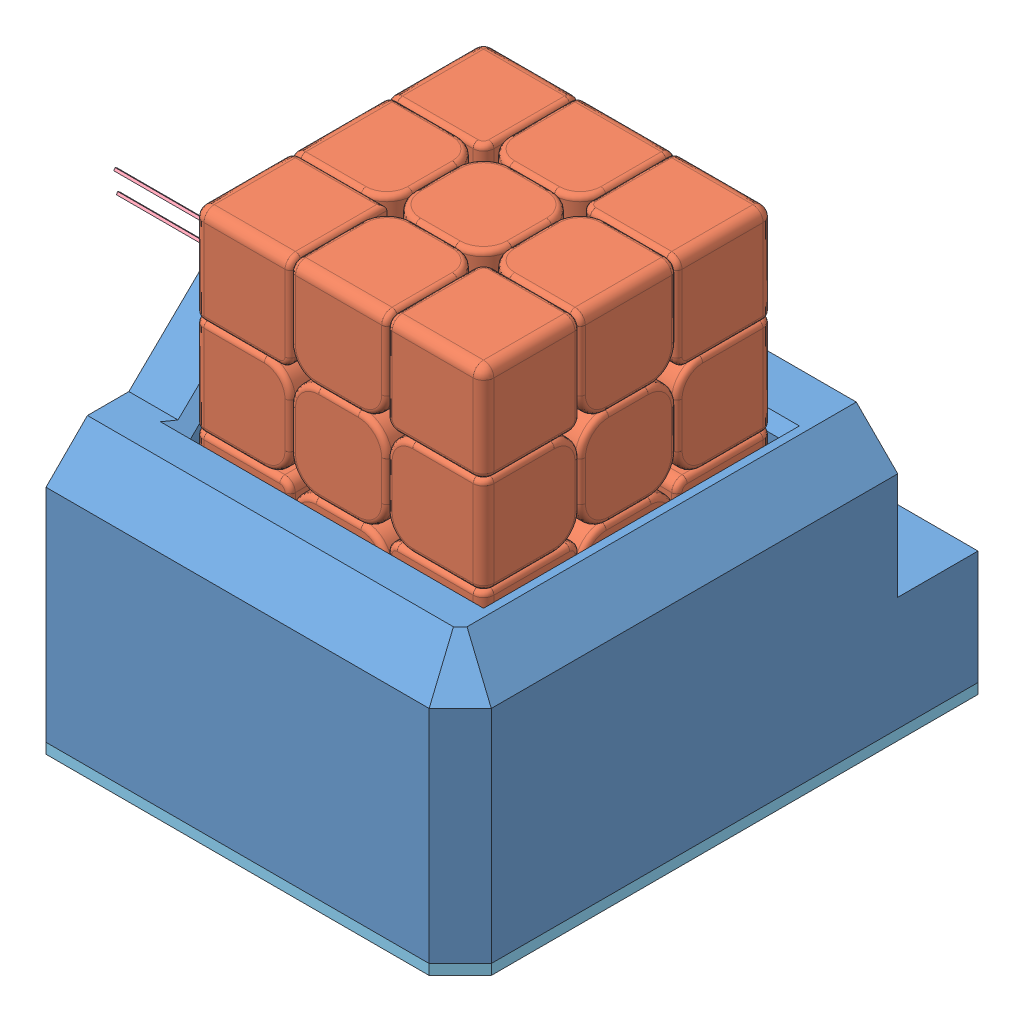
SolidWorks assembly Color Scanner Assembly, configuration Default. Lengths in mm.
Overall size (113 101.69 100).
24 component instances, 5 part files, 54 mates.
Components (placement in the parent):
- Color Scanner Base-1: Color Scanner Base [Default] at (-49.0909 -2.3854 18.9197) size (80 69.33 100)
- Cube-1: Cube [Default] at (-49.0909 35.3042 24.4197) size (56 56 56)
- Universal_board_70x90mm_Defeatured-1: Universal_board_70x90mm_Defeatured [Default] at (-130.3648 -15.8854 -34.2522) size (70 1.6 90)
- LED 5mm-1: LED 5mm [Valor predeterminado] at (-71.5909 -6.3854 24.4197) x (-0.837169 0 -0.546944) z (0 1 0) size (10.06 6 40.8)
- LED 5mm-2: LED 5mm [Valor predeterminado] at (-34.2576 -6.3854 5.753) x (-0.837169 0 -0.546944) z (0 1 0) size (10.06 6 40.8)
- LED 5mm-3: LED 5mm [Valor predeterminado] at (-63.9242 -6.3854 24.4197) x (-0.837169 0 -0.546944) z (0 1 0) size (10.06 6 40.8)
- LED 5mm-4: LED 5mm [Valor predeterminado] at (-52.9242 -6.3854 24.4197) x (-0.837169 0 -0.546944) z (0 1 0) size (10.06 6 40.8)
- LED 5mm-5: LED 5mm [Valor predeterminado] at (-63.9242 -6.3854 5.753) x (-0.837169 0 -0.546944) z (0 1 0) size (10.06 6 40.8)
- LED 5mm-6: LED 5mm [Valor predeterminado] at (-71.5909 -6.3854 5.753) x (-0.930459 0 -0.366395) z (0 1 0) size (10.06 6 40.8)
- LED 5mm-7: LED 5mm [Valor predeterminado] at (-45.2576 -6.3854 5.753) x (-0.837169 0 -0.546944) z (0 1 0) size (10.06 6 40.8)
- LED 5mm-8: LED 5mm [Valor predeterminado] at (-52.9242 -6.3854 5.753) x (-0.837169 0 -0.546944) z (0 1 0) size (10.06 6 40.8)
- LED 5mm-9: LED 5mm [Valor predeterminado] at (-45.2576 -6.3854 24.4197) x (-0.837169 0 -0.546944) z (0 1 0) size (10.06 6 40.8)
- LED 5mm-10: LED 5mm [Valor predeterminado] at (-34.2576 -6.3854 43.0863) x (-0.837169 0 -0.546944) z (0 1 0) size (10.06 6 40.8)
- LED 5mm-11: LED 5mm [Valor predeterminado] at (-26.5909 -6.3854 5.753) x (-0.837169 0 -0.546944) z (0 1 0) size (10.06 6 40.8)
- LED 5mm-12: LED 5mm [Valor predeterminado] at (-45.2576 -6.3854 43.0863) x (-0.837169 0 -0.546944) z (0 1 0) size (10.06 6 40.8)
- LED 5mm-13: LED 5mm [Valor predeterminado] at (-26.5909 -6.3854 43.0863) x (-0.837169 0 -0.546944) z (0 1 0) size (10.06 6 40.8)
- LED 5mm-14: LED 5mm [Valor predeterminado] at (-71.5909 -6.3854 43.0863) x (-0.837169 0 -0.546944) z (0 1 0) size (10.06 6 40.8)
- LED 5mm-15: LED 5mm [Valor predeterminado] at (-26.5909 -6.3854 24.4197) x (-0.837169 0 -0.546944) z (0 1 0) size (10.06 6 40.8)
- LED 5mm-16: LED 5mm [Valor predeterminado] at (-52.9242 -6.3854 43.0863) x (-0.837169 0 -0.546944) z (0 1 0) size (10.06 6 40.8)
- LED 5mm-17: LED 5mm [Valor predeterminado] at (-34.2576 -6.3854 24.4197) x (-0.837169 0 -0.546944) z (0 1 0) size (10.06 6 40.8)
- LED 5mm-18: LED 5mm [Valor predeterminado] at (-63.9242 -6.3854 43.0863) x (-0.837169 0 -0.546944) z (0 1 0) size (10.06 6 40.8)
- LED 5mm-20: LED 5mm [Valor predeterminado] at (-90.0909 35.6146 28.253) x (0 0.837169 -0.546944) z (1 0 0) size (10.06 6 40.8)
- LED 5mm-21: LED 5mm [Valor predeterminado] at (-90.0909 35.6146 20.5863) x (0 0.837169 -0.546944) z (1 0 0) size (10.06 6 40.8)
- Color Sensor Baseplate-1: Color Sensor Baseplate [Default] at (-49.0909 -24.3854 18.9197) x (1 0 0) z (0 0 -1) size (80 8.5 100)
Mates (geometry in assembly coordinates):
- Width1: width anti-aligned: plane of Color Scanner Base-1 through (-77.5909 26.2812 18.9197) normal (1 0 0); plane of Cube-1 through (-20.5909 26.2812 18.9197) normal (-1 0 0); plane of Color Scanner Base-1 through (-77.0909 7.3042 52.4197) normal (-1 0 0); plane of Cube-1 through (-21.0909 7.3042 52.4197) normal (1 0 0)
- Width2: width anti-aligned: plane of Color Scanner Base-1 through (-49.0909 26.2812 52.9197) normal (0 0 -1); plane of Cube-1 through (-49.0909 26.2812 -4.0803) normal (0 0 1); plane of Color Scanner Base-1 through (-77.0909 7.3042 52.4197) normal (0 0 1); plane of Cube-1 through (-77.0909 7.3042 -3.5803) normal (0 0 -1)
- Coincident3: coincident anti-aligned: plane of Color Scanner Base-1 through (-84.5909 -14.3854 -26.5803) normal (0 -1 0); plane of Universal_board_70x90mm_Defeatured-1 through (-91.0909 -14.3854 72.9197) normal (0 1 0)
- Width3: width anti-aligned: plane of Color Scanner Base-1 through (-84.5909 113.0355 -26.5803) normal (1 0 0); plane of Universal_board_70x90mm_Defeatured-1 through (-13.5909 113.0355 -26.5803) normal (-1 0 0); plane of Color Scanner Base-1 through (-84.0909 -16.0354 72.9197) normal (-1 0 0); plane of Universal_board_70x90mm_Defeatured-1 through (-14.0909 -14.2354 72.9197) normal (1 0 0)
- Width4: width anti-aligned: plane of Universal_board_70x90mm_Defeatured-1 through (-91.0909 -14.2354 63.9197) normal (0 0 1); plane of Color Scanner Base-1 through (-91.0909 -16.0354 -26.0803) normal (0 0 -1); plane of Universal_board_70x90mm_Defeatured-1 through (-84.5909 113.0355 64.4197) normal (0 0 -1); plane of Color Scanner Base-1 through (-84.5909 113.0355 -26.5803) normal (0 0 1)
- Concentric2: concentric aligned: cylinder of Color Scanner Base-1 through (-71.5909 26.2812 5.753) axis (0 -1 0) radius 2.75; cylinder of LED 5mm-6 through (-71.5909 -5.3854 5.753) axis (0 -1 0) radius 2.5
- Coincident6: coincident aligned: plane of Color Scanner Base-1 through (-49.0909 -6.3854 18.9197) normal (0 -1 0); plane of LED 5mm-6 through (-71.5909 -6.3854 5.753) normal (0 -1 0)
- Concentric4: concentric aligned: cylinder of Color Scanner Base-1 through (-63.9242 26.2812 5.753) axis (0 -1 0) radius 2.75; cylinder of LED 5mm-5 through (-63.9242 -5.3854 5.753) axis (0 -1 0) radius 2.5
- Coincident7: coincident aligned: plane of Color Scanner Base-1 through (-49.0909 -6.3854 18.9197) normal (0 -1 0); plane of LED 5mm-5 through (-63.9242 -6.3854 5.753) normal (0 -1 0)
- Concentric6: concentric aligned: cylinder of Color Scanner Base-1 through (-52.9242 26.2812 5.753) axis (0 -1 0) radius 2.75; cylinder of LED 5mm-8 through (-52.9242 -5.3854 5.753) axis (0 -1 0) radius 2.5
- Concentric7: concentric aligned: cylinder of Color Scanner Base-1 through (-45.2576 26.2812 5.753) axis (0 -1 0) radius 2.75; cylinder of LED 5mm-7 through (-45.2576 -5.3854 5.753) axis (0 -1 0) radius 2.5
- Coincident8: coincident aligned: plane of Color Scanner Base-1 through (-49.0909 -6.3854 18.9197) normal (0 -1 0); plane of LED 5mm-8 through (-52.9242 -6.3854 5.753) normal (0 -1 0)
- Coincident9: coincident aligned: plane of Color Scanner Base-1 through (-49.0909 -6.3854 18.9197) normal (0 -1 0); plane of LED 5mm-7 through (-45.2576 -6.3854 5.753) normal (0 -1 0)
- Concentric8: concentric aligned: cylinder of Color Scanner Base-1 through (-34.2576 26.2812 5.753) axis (0 -1 0) radius 2.75; cylinder of LED 5mm-2 through (-34.2576 -5.3854 5.753) axis (0 -1 0) radius 2.5
- Coincident10: coincident aligned: plane of Color Scanner Base-1 through (-49.0909 -6.3854 18.9197) normal (0 -1 0); plane of LED 5mm-2 through (-34.2576 -6.3854 5.753) normal (0 -1 0)
- Concentric9: concentric aligned: cylinder of Color Scanner Base-1 through (-26.5909 26.2812 5.753) axis (0 -1 0) radius 2.75; cylinder of LED 5mm-11 through (-26.5909 -5.3854 5.753) axis (0 -1 0) radius 2.5
- Coincident11: coincident aligned: plane of Color Scanner Base-1 through (-49.0909 -6.3854 18.9197) normal (0 -1 0); plane of LED 5mm-11 through (-26.5909 -6.3854 5.753) normal (0 -1 0)
- Concentric10: concentric aligned: cylinder of Color Scanner Base-1 through (-71.5909 26.2812 24.4197) axis (0 -1 0) radius 2.75; cylinder of LED 5mm-1 through (-71.5909 -5.3854 24.4197) axis (0 -1 0) radius 2.5
- Concentric11: concentric aligned: cylinder of Color Scanner Base-1 through (-63.9242 26.2812 24.4197) axis (0 -1 0) radius 2.75; cylinder of LED 5mm-3 through (-63.9242 -5.3854 24.4197) axis (0 -1 0) radius 2.5
- Concentric12: concentric aligned: cylinder of Color Scanner Base-1 through (-52.9242 26.2812 24.4197) axis (0 -1 0) radius 2.75; cylinder of LED 5mm-4 through (-52.9242 -5.3854 24.4197) axis (0 -1 0) radius 2.5
- Coincident12: coincident aligned: plane of Color Scanner Base-1 through (-49.0909 -6.3854 18.9197) normal (0 -1 0); plane of LED 5mm-3 through (-63.9242 -6.3854 24.4197) normal (0 -1 0)
- Coincident13: coincident aligned: plane of Color Scanner Base-1 through (-49.0909 -6.3854 18.9197) normal (0 -1 0); plane of LED 5mm-4 through (-52.9242 -6.3854 24.4197) normal (0 -1 0)
- Concentric13: concentric aligned: cylinder of Color Scanner Base-1 through (-45.2576 26.2812 24.4197) axis (0 -1 0) radius 2.75; cylinder of LED 5mm-9 through (-45.2576 -5.3854 24.4197) axis (0 -1 0) radius 2.5
- Concentric15: concentric aligned: cylinder of Color Scanner Base-1 through (-34.2576 26.2812 24.4197) axis (0 -1 0) radius 2.75; cylinder of LED 5mm-17 through (-34.2576 -5.3854 24.4197) axis (0 -1 0) radius 2.5
- Concentric16: concentric aligned: cylinder of Color Scanner Base-1 through (-26.5909 26.2812 24.4197) axis (0 -1 0) radius 2.75; cylinder of LED 5mm-15 through (-26.5909 -5.3854 24.4197) axis (0 -1 0) radius 2.5
- Concentric17: concentric aligned: cylinder of Color Scanner Base-1 through (-26.5909 26.2812 43.0863) axis (0 -1 0) radius 2.75; cylinder of LED 5mm-13 through (-26.5909 -5.3854 43.0863) axis (0 -1 0) radius 2.5
- Concentric18: concentric aligned: cylinder of Color Scanner Base-1 through (-34.2576 26.2812 43.0863) axis (0 -1 0) radius 2.75; cylinder of LED 5mm-10 through (-34.2576 -5.3854 43.0863) axis (0 -1 0) radius 2.5
- Concentric19: concentric aligned: cylinder of Color Scanner Base-1 through (-45.2576 26.2812 43.0863) axis (0 -1 0) radius 2.75; cylinder of LED 5mm-12 through (-45.2576 -5.3854 43.0863) axis (0 -1 0) radius 2.5
- Concentric20: concentric aligned: cylinder of Color Scanner Base-1 through (-52.9242 26.2812 43.0863) axis (0 -1 0) radius 2.75; cylinder of LED 5mm-16 through (-52.9242 -5.3854 43.0863) axis (0 -1 0) radius 2.5
- Concentric21: concentric aligned: cylinder of Color Scanner Base-1 through (-63.9242 26.2812 43.0863) axis (0 -1 0) radius 2.75; cylinder of LED 5mm-18 through (-63.9242 -5.3854 43.0863) axis (0 -1 0) radius 2.5
- Concentric22: concentric aligned: cylinder of Color Scanner Base-1 through (-71.5909 26.2812 43.0863) axis (0 -1 0) radius 2.75; cylinder of LED 5mm-14 through (-71.5909 -5.3854 43.0863) axis (0 -1 0) radius 2.5
- Coincident14: coincident aligned: plane of Color Scanner Base-1 through (-49.0909 -6.3854 18.9197) normal (0 -1 0); plane of LED 5mm-1 through (-71.5909 -6.3854 24.4197) normal (0 -1 0)
- Coincident15: coincident aligned: plane of Color Scanner Base-1 through (-49.0909 -6.3854 18.9197) normal (0 -1 0); plane of LED 5mm-6 through (-71.5909 -6.3854 5.753) normal (0 -1 0)
- Coincident16: coincident aligned: plane of Color Scanner Base-1 through (-49.0909 -6.3854 18.9197) normal (0 -1 0); plane of LED 5mm-5 through (-63.9242 -6.3854 5.753) normal (0 -1 0)
- Coincident17: coincident aligned: plane of Color Scanner Base-1 through (-49.0909 -6.3854 18.9197) normal (0 -1 0); plane of LED 5mm-8 through (-52.9242 -6.3854 5.753) normal (0 -1 0)
- Coincident18: coincident aligned: plane of Color Scanner Base-1 through (-49.0909 -6.3854 18.9197) normal (0 -1 0); plane of LED 5mm-7 through (-45.2576 -6.3854 5.753) normal (0 -1 0)
- Coincident19: coincident aligned: plane of Color Scanner Base-1 through (-49.0909 -6.3854 18.9197) normal (0 -1 0); plane of LED 5mm-2 through (-34.2576 -6.3854 5.753) normal (0 -1 0)
- Coincident20: coincident aligned: plane of Color Scanner Base-1 through (-49.0909 -6.3854 18.9197) normal (0 -1 0); plane of LED 5mm-11 through (-26.5909 -6.3854 5.753) normal (0 -1 0)
- Coincident21: coincident aligned: plane of Color Scanner Base-1 through (-49.0909 -6.3854 18.9197) normal (0 -1 0); plane of LED 5mm-17 through (-34.2576 -6.3854 24.4197) normal (0 -1 0)
- Coincident22: coincident aligned: plane of Color Scanner Base-1 through (-49.0909 -6.3854 18.9197) normal (0 -1 0); plane of LED 5mm-15 through (-26.5909 -6.3854 24.4197) normal (0 -1 0)
- Coincident23: coincident aligned: plane of Color Scanner Base-1 through (-49.0909 -6.3854 18.9197) normal (0 -1 0); plane of LED 5mm-14 through (-71.5909 -6.3854 43.0863) normal (0 -1 0)
- Coincident24: coincident aligned: plane of Color Scanner Base-1 through (-49.0909 -6.3854 18.9197) normal (0 -1 0); plane of LED 5mm-18 through (-63.9242 -6.3854 43.0863) normal (0 -1 0)
- Coincident25: coincident aligned: plane of Color Scanner Base-1 through (-49.0909 -6.3854 18.9197) normal (0 -1 0); plane of LED 5mm-16 through (-52.9242 -6.3854 43.0863) normal (0 -1 0)
- Coincident26: coincident aligned: plane of Color Scanner Base-1 through (-49.0909 -6.3854 18.9197) normal (0 -1 0); plane of LED 5mm-12 through (-45.2576 -6.3854 43.0863) normal (0 -1 0)
- Coincident27: coincident aligned: plane of Color Scanner Base-1 through (-49.0909 -6.3854 18.9197) normal (0 -1 0); plane of LED 5mm-10 through (-34.2576 -6.3854 43.0863) normal (0 -1 0)
- Coincident28: coincident aligned: plane of Color Scanner Base-1 through (-49.0909 -6.3854 18.9197) normal (0 -1 0); plane of LED 5mm-13 through (-26.5909 -6.3854 43.0863) normal (0 -1 0)
- Coincident29: coincident aligned: plane of Color Scanner Base-1 through (-49.0909 -6.3854 18.9197) normal (0 -1 0); plane of LED 5mm-9 through (-45.2576 -6.3854 24.4197) normal (0 -1 0)
- Concentric23: concentric anti-aligned: cylinder of Color Scanner Base-1 through (-89.0909 35.6146 28.253) axis (1 0 0) radius 2.5; cylinder of LED 5mm-20 through (-89.0909 35.6146 28.253) axis (-1 0 0) radius 2.5
- Concentric24: concentric anti-aligned: cylinder of Color Scanner Base-1 through (-89.0909 35.6146 20.5863) axis (1 0 0) radius 2.5; cylinder of LED 5mm-21 through (-89.0909 35.6146 20.5863) axis (-1 0 0) radius 2.5
- Coincident30: coincident anti-aligned: plane of Color Scanner Base-1 through (-89.0909 -24.3854 68.9197) normal (-1 0 0); plane of LED 5mm-21 through (-89.0909 35.6146 20.5863) normal (1 0 0)
- Coincident31: coincident anti-aligned: plane of Color Scanner Base-1 through (-89.0909 -24.3854 68.9197) normal (-1 0 0); plane of LED 5mm-20 through (-89.0909 35.6146 28.253) normal (1 0 0)
- Coincident35: coincident anti-aligned: plane of Color Scanner Base-1 through (-49.0909 -24.3854 18.9197) normal (0 -1 0); plane of Color Sensor Baseplate-1 through (-49.0909 -24.3854 18.9197) normal (0 1 0)
- Coincident36: coincident aligned: plane of Color Scanner Base-1 through (-15.0909 -24.3854 68.9197) normal (0.707107 0 0.707107); plane of Color Sensor Baseplate-1 through (-15.0909 -26.3854 68.9197) normal (0.707107 0 0.707107)
- Coincident37: coincident aligned: plane of Color Scanner Base-1 through (-9.0909 -24.3854 68.9197) normal (1 0 0); plane of Color Sensor Baseplate-1 through (-9.0909 -26.3854 68.9197) normal (1 0 0)
